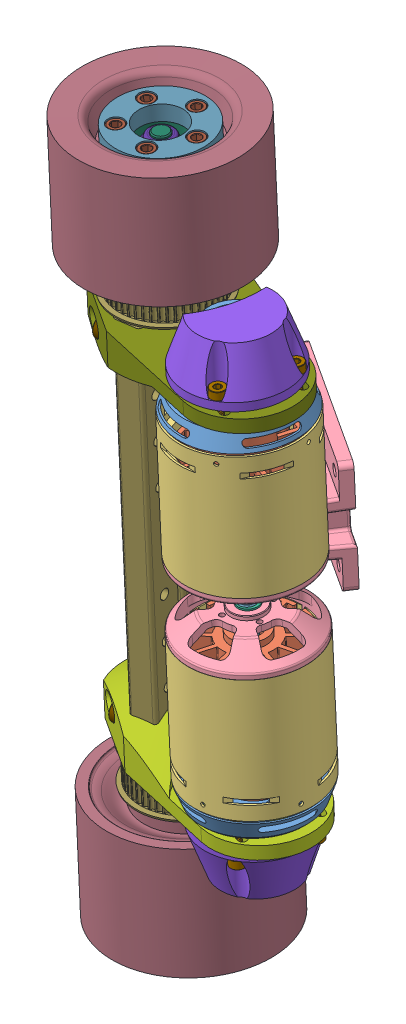
SolidWorks assembly MBS trucks, configuration Default. Lengths in mm.
Overall size (186.8 351.93 169.98).
89 component instances, 34 part files, 94 mates.
Components (placement in the parent):
- GPA26GT3150-A-N8-2: GPA26GT3150-A-N8 [Default] at (26.5522 -42.4742 -58.9865) x (-0.019038 0.999391 0.029249) z (0.77019 0.033313 -0.636944) size (20 28 28)
  - GPA26GT3150-A-N8_b-1: GPA26GT3150-A-N8_b [Default] at origin size (20 28 28)
  - SET-SCREW4-3-1: SET-SCREW4-3 [Default] at (10 5.4 0) x (0 -1 0) z (-1 0 0) size (3 4 4)
  - SET-SCREW4-3-2: SET-SCREW4-3 [Default] at (10 -2.2723 -3.2919) x (0 0.568065 0.822984) z (-1 0 0) size (3 4 4)
- Key20mm-2: Key20mm [Default] at (29.2375 -42.4492 -58.093) x (-0.77019 -0.033313 0.636944) z (-0.63753 0.010401 -0.770355) size (3 20 3)
- MarkIITrucksCustomHanger-1: MarkIITrucksCustomHanger [Default] at (-31.1638 36.2817 -181.4556) x (-0.019038 0.999391 0.029249) z (0.838104 0 0.54551) size (348 118.71 110.67)
  - 50cal_baseplateEDIT-1: 50cal_baseplateEDIT [Default] at (40.8754 28.4427 48.4148) size (55.88 41.6 78.53)
  - BS_bushing-1: BS_bushing [Default] at (40.8754 74.2758 55.8381) x (0.903515 -0.328294 -0.275471) z (-0.428557 -0.692132 -0.580768) size (24.64 14.73 24.64)
  - BS_washer-1: BS_washer [Default] at (40.8754 63.8267 68.2909) x (0.781233 0.478195 0.401253) z (-0.624239 0.59846 0.502167) size (29.08 4.06 29.08)
  - kingpin-1: kingpin [Default] at (40.8754 51.905 82.4986) x (0.057682 0.764769 0.641717) z (0.998335 -0.044187 -0.037077) size (16.06 70.1 13.91)
  - kingpin-nut-1: kingpin-nut [90630A115] at (40.8754 87.1097 40.5433) x (0.976709 0.16437 0.137923) z (-0.214569 0.748202 0.627816) size (12.7 8.97 14.66)
  - Pivot_cup-1: Pivot_cup [Default] at (40.8754 44.9216 26.2393) x (-0.987309 0.102082 -0.121656) z (0.158811 0.63463 -0.756323) size (17.46 19.05 17.46)
  - RS_bushing-1: RS_bushing [Default] at (40.8754 76.7422 52.8988) x (0.999722 0.018072 0.015164) z (-0.023591 0.765831 0.642609) size (24.77 14.61 24.77)
  - washer-1: washer [Default] at (171.3754 88.007 62.3923) x (0 0.98686 -0.161575) z (0 0.161575 0.98686) size (11 1 11)
  - BS_washer-2: BS_washer [Default] at (40.8754 87.1097 40.5433) x (-0.947616 0.244683 0.205314) z (0.319411 0.725916 0.609116) size (29.08 4.06 29.08)
  - washer-2: washer [Default] at (196.6254 88.007 62.3923) x (0 -0.726217 0.687466) z (0 -0.687466 -0.726217) size (11 1 11)
  - CustomHanger-1: CustomHanger [Default] at (40.8754 81.1126 56.6072) x (1 0 0) z (0 -0.642788 0.766044) size (253 93.96 18)
  - KegelWheelAssembly-1: KegelWheelAssembly [Default] at (208.2287 131.5766 17.5506) x (0 0.867364 -0.497674) z (0 0.497674 0.867364) size (80 56 80)
    - Kegel 80mm longboard wheel-1: Kegel 80mm longboard wheel [Default] at (-60.1073 30.6906 17.2106) size (80 56 80)
    - 608-bearing-1: 608-bearing [6661K82] at (-60.1073 32.8534 17.2106) x (1 0 0) z (0 -1 0) size (22 22 7)
    - 608-bearing-2: 608-bearing [6661K82] at (-60.1073 15.6034 17.2106) x (-0.561464 0 0.827501) z (0 -1 0) size (22 22 7)
  - FPSSFJAD-D10-L64-T36-Q8-1: FPSSFJAD-D10-L64-T36-Q8 [Default] at (106.8754 88.007 62.3923) x (1 0 0) z (0 -0.232371 0.972627) size (100 10 10)
  - SetScrew_SAE_10-32x.5in-1: SetScrew_SAE_10-32x.5in [92313A829] at (130.8754 96.8695 69.8289) x (0.758718 0.418725 -0.499016) z (0 0.766044 0.642788) size (4.96 4.83 13.07)
  - SetScrew_SAE_10-32x.5in-3: SetScrew_SAE_10-32x.5in [92313A829] at (130.8736 79.1457 54.9542) x (0.758718 0.418725 -0.499016) z (0 -0.766044 -0.642788) size (4.96 4.83 13.07)
  - NylonLockNut_5.16-24-1: NylonLockNut_5.16-24 [97135A225] at (197.1254 88.007 62.3923) x (0 0.323657 0.946174) z (0 0.946174 -0.323657) size (12.7 8.97 14.66)
  - KegelWheelAssembly-3: KegelWheelAssembly [Default] at (-126.478 148.7071 47.4063) x (0 0.867364 -0.497674) z (0 -0.497674 -0.867364) size (80 56 80)
    - Kegel 80mm longboard wheel-1: Kegel 80mm longboard wheel [Default] at (-60.1073 30.6906 17.2106) size (80 56 80)
    - 608-bearing-1: 608-bearing [6661K82] at (-60.1073 32.8534 17.2106) x (1 0 0) z (0 -1 0) size (22 22 7)
    - 608-bearing-2: 608-bearing [6661K82] at (-60.1073 15.6034 17.2106) x (-0.561464 0 0.827501) z (0 -1 0) size (22 22 7)
  - FPSSFJAD-D10-L64-T36-Q8-3: FPSSFJAD-D10-L64-T36-Q8 [Default] at (-25.1246 88.007 62.3923) x (-1 0 0) z (0 0.232371 -0.972627) size (100 10 10)
  - NylonLockNut_5.16-24-3: NylonLockNut_5.16-24 [97135A225] at (-115.3746 88.007 62.3923) x (0 -0.323657 -0.946174) z (0 0.946174 -0.323657) size (12.7 8.97 14.66)
  - SetScrew_SAE_10-32x.5in-7: SetScrew_SAE_10-32x.5in [92313A829] at (-49.1228 96.8708 69.8273) x (-0.758718 0.418725 -0.499016) z (0 0.766044 0.642788) size (4.96 4.83 13.07)
  - SetScrew_SAE_10-32x.5in-8: SetScrew_SAE_10-32x.5in [92313A829] at (-49.1246 79.1444 54.9557) x (-0.758718 0.418725 -0.499016) z (0 -0.766044 -0.642788) size (4.96 4.83 13.07)
- 91274A172_COATED ALLOY STEEL SOCKET HEAD CAP SCREW-1: 91274A172_COATED ALLOY STEEL SOCKET HEAD CAP SCREW [91274A172] at (-10.1778 -9.516 -60.2635) x (0.117443 0.107613 0.987232) z (0.992459 0.022433 -0.12051) size (9.53 9.53 32.48)
- 91274A172_COATED ALLOY STEEL SOCKET HEAD CAP SCREW-2: 91274A172_COATED ALLOY STEEL SOCKET HEAD CAP SCREW [91274A172] at (-14.1739 -8.6338 -93.0088) x (-0.014856 -0.953854 -0.299902) z (0.992459 0.022433 -0.12051) size (9.53 9.53 32.48)
- 91274A172_COATED ALLOY STEEL SOCKET HEAD CAP SCREW-7: 91274A172_COATED ALLOY STEEL SOCKET HEAD CAP SCREW [91274A172] at (-13.3571 157.3822 -55.3789) x (-0.122553 0.160599 -0.979382) z (0.992459 0.022433 -0.12051) size (9.53 9.53 32.48)
- Turnigy6374-6: Turnigy6374 [Default] at (18.5878 -4.184 -56.238) x (0.309684 0.03371 -0.950242) z (-0.950649 -0.009033 -0.310137) size (83.4 113.65 83.4)
  - Stator-1: Stator [Default] at (3.7873 1.8989 -6.3731) size (58.75 9.22 58.75)
  - StatorPart2-1: StatorPart2 [Default] at (3.7873 -16.3511 -6.3731) size (50 66 50)
  - AxelHoldCover-1: AxelHoldCover [Default] at (3.7873 -60.8511 -6.3731) x (0.982235 0 -0.187653) z (0.187653 0 0.982235) size (59.15 61.5 59.15)
  - AxelHold-1: AxelHold [Default] at (3.7873 -60.8511 -6.3731) x (0.729158 0 0.684345) z (0.684345 0 -0.729158) size (59 18.5 59)
  - AxisCust-1: AxisCust [Default] at (3.7873 -73.3511 -6.3731) x (0.844889 0 -0.534942) z (0.534942 0 0.844889) size (8 113.65 8)
  - 90967A120_STAINLESS STEEL EXTERNAL RETAINING RING-1: 90967A120_STAINLESS STEEL EXTERNAL RETAINING RING [90967A120] at (3.7873 12.2489 -6.3731) x (0 -1 0) z (0 0 1) size (0.8 12.1 9.85)
  - 90967A120_STAINLESS STEEL EXTERNAL RETAINING RING-2: 90967A120_STAINLESS STEEL EXTERNAL RETAINING RING [90967A120] at (3.7873 -73.7511 -6.3731) x (0 -1 0) z (-0.841191 0 -0.540738) size (0.8 12.1 9.85)
- MotorMountLeft-3: MotorMountLeft [Default] at (-25.8025 -21.8807 -75.3183) x (-0.019038 0.999391 0.029249) z (-0.309684 -0.03371 0.950242) size (25.4 116.05 69.01)
- Belt Cap Wheel Side - Motor-2: Belt Cap Wheel Side - Motor [Default] at (26.1505 -21.387 -58.3693) x (-0.309684 -0.03371 0.950242) z (0.950649 0.009033 0.310137) size (50.8 25 40.64)
- M4x16mm_BlackZincSteel-3: M4x16mm_BlackZincSteel [91274A119] at (45.5282 -8.7294 -67.976) x (0.992084 0.022514 -0.123538) z (-0.019038 0.999391 0.029249) size (7 7 20.35)
- M4x16mm_BlackZincSteel-4: M4x16mm_BlackZincSteel [91274A119] at (35.8931 -9.7782 -38.4114) x (0.992084 0.022514 -0.123538) z (-0.019038 0.999391 0.029249) size (7 7 20.35)
- 92125A192_TYPE 18-8 SS FLAT-HEAD SOCKET CAP SCREW-9: 92125A192_TYPE 18-8 SS FLAT-HEAD SOCKET CAP SCREW [92125A192] at (16.1756 -20.8033 -77.9703) x (-0.507945 -0.034866 0.860683) z (0.019038 -0.999391 -0.029249) size (8 8 12.4)
- 92125A192_TYPE 18-8 SS FLAT-HEAD SOCKET CAP SCREW-10: 92125A192_TYPE 18-8 SS FLAT-HEAD SOCKET CAP SCREW [92125A192] at (6.5405 -21.8521 -48.4057) x (0.99191 0.022552 -0.124927) z (0.019038 -0.999391 -0.029249) size (8 8 12.4)
- 91251A355_BLACK-OXIDE ALLOY STEEL SOCKET HEAD CAP SCREW-11: 91251A355_BLACK-OXIDE ALLOY STEEL SOCKET HEAD CAP SCREW [91251A355] at (-23.2576 -26.4129 -91.1172) x (0.999816 0.019099 -0.00181) z (-0.019038 0.999391 0.029249) size (7.92 7.92 68.91)
- GPA50GT3150-A-H26_b-1: GPA50GT3150-A-H26_b [Default] at (-25.7787 -23.1299 -75.3548) x (0.019038 -0.999391 -0.029249) z (0.987808 0.01428 0.155018) size (20 51 51)
- Wheel Spacer 2-3: Wheel Spacer 2 [Default] at (-25.0284 -62.5187 -76.5076) x (-0.158306 0.025873 -0.987051) z (0.987207 0.023422 -0.157717) size (44 14.02 44)
- Wheel Spacer Alum-3: Wheel Spacer Alum [Default] at (-25.0284 -62.5187 -76.5076) x (-0.158306 0.025873 -0.987051) z (0.987207 0.023422 -0.157717) size (44 7.62 44)
- 91251A355_BLACK-OXIDE ALLOY STEEL SOCKET HEAD CAP SCREW-12: 91251A355_BLACK-OXIDE ALLOY STEEL SOCKET HEAD CAP SCREW [91251A355] at (-39.8403 -26.9769 -82.6391) x (0.306709 0.033682 -0.951207) z (-0.019038 0.999391 0.029249) size (7.92 7.92 68.91)
- 91251A355_BLACK-OXIDE ALLOY STEEL SOCKET HEAD CAP SCREW-13: 91251A355_BLACK-OXIDE ALLOY STEEL SOCKET HEAD CAP SCREW [91251A355] at (-36.8906 -27.459 -64.2475) x (-0.81026 0.001717 -0.586069) z (-0.019038 0.999391 0.029249) size (7.92 7.92 68.91)
- 91251A355_BLACK-OXIDE ALLOY STEEL SOCKET HEAD CAP SCREW-14: 91251A355_BLACK-OXIDE ALLOY STEEL SOCKET HEAD CAP SCREW [91251A355] at (-18.485 -27.1929 -61.3591) x (-0.807477 -0.03262 0.588997) z (-0.019038 0.999391 0.029249) size (7.92 7.92 68.91)
- 91251A355_BLACK-OXIDE ALLOY STEEL SOCKET HEAD CAP SCREW-15: 91251A355_BLACK-OXIDE ALLOY STEEL SOCKET HEAD CAP SCREW [91251A355] at (-10.0593 -26.5464 -77.9655) x (0.311212 -0.021878 0.950089) z (-0.019038 0.999391 0.029249) size (7.92 7.92 68.91)
- Wheel Spacer-3: Wheel Spacer [Default] at (-25.0284 -62.5187 -76.5076) x (0.154506 0.031844 -0.987479) z (0.987808 0.01428 0.155018) size (44 7.02 44)
- 91274A172_COATED ALLOY STEEL SOCKET HEAD CAP SCREW-8: 91274A172_COATED ALLOY STEEL SOCKET HEAD CAP SCREW [91274A172] at (-13.3571 157.3822 -55.3789) x (-0.122553 0.160599 -0.979382) z (0.992459 0.022433 -0.12051) size (9.53 9.53 32.48)
- 91274A172_COATED ALLOY STEEL SOCKET HEAD CAP SCREW-9: 91274A172_COATED ALLOY STEEL SOCKET HEAD CAP SCREW [91274A172] at (-17.3532 158.2645 -88.1242) x (0.051476 -0.968499 0.24364) z (0.992459 0.022433 -0.12051) size (9.53 9.53 32.48)
- Turnigy6374-7: Turnigy6374 [Default] at (27.7121 153.0376 -47.6869) x (0.309684 0.03371 -0.950242) z (0.950649 0.009033 0.310137) size (83.4 113.65 83.4)
  - Stator-1: Stator [Default] at (3.7873 1.8989 -6.3731) size (58.75 9.22 58.75)
  - StatorPart2-1: StatorPart2 [Default] at (3.7873 -16.3511 -6.3731) size (50 66 50)
  - AxelHoldCover-1: AxelHoldCover [Default] at (3.7873 -60.8511 -6.3731) x (0.982235 0 -0.187653) z (0.187653 0 0.982235) size (59.15 61.5 59.15)
  - AxelHold-1: AxelHold [Default] at (3.7873 -60.8511 -6.3731) x (0.729158 0 0.684345) z (0.684345 0 -0.729158) size (59 18.5 59)
  - AxisCust-1: AxisCust [Default] at (3.7873 -73.3511 -6.3731) x (0.844889 0 -0.534942) z (0.534942 0 0.844889) size (8 113.65 8)
  - 90967A120_STAINLESS STEEL EXTERNAL RETAINING RING-1: 90967A120_STAINLESS STEEL EXTERNAL RETAINING RING [90967A120] at (3.7873 12.2489 -6.3731) x (0 -1 0) z (0 0 1) size (0.8 12.1 9.85)
  - 90967A120_STAINLESS STEEL EXTERNAL RETAINING RING-2: 90967A120_STAINLESS STEEL EXTERNAL RETAINING RING [90967A120] at (3.7873 -73.7511 -6.3731) x (0 -1 0) z (-0.841191 0 -0.540738) size (0.8 12.1 9.85)
- Belt Cap Wheel Side - Motor-3: Belt Cap Wheel Side - Motor [Default] at (22.4952 170.496 -52.7534) x (0.309684 0.03371 -0.950242) z (0.950649 0.009033 0.310137) size (50.8 25 40.64)
- M4x16mm_BlackZincSteel-5: M4x16mm_BlackZincSteel [91274A119] at (42.3298 159.1682 -63.0621) x (0.992084 0.022514 -0.123538) z (0.019038 -0.999391 -0.029249) size (7 7 20.35)
- M4x16mm_BlackZincSteel-6: M4x16mm_BlackZincSteel [91274A119] at (32.6947 158.1194 -33.4975) x (0.992084 0.022514 -0.123538) z (0.019038 -0.999391 -0.029249) size (7 7 20.35)
- 92125A192_TYPE 18-8 SS FLAT-HEAD SOCKET CAP SCREW-11: 92125A192_TYPE 18-8 SS FLAT-HEAD SOCKET CAP SCREW [92125A192] at (12.5279 170.68 -72.3661) x (0.507945 0.034866 -0.860683) z (-0.019038 0.999391 0.029249) size (8 8 12.4)
- 92125A192_TYPE 18-8 SS FLAT-HEAD SOCKET CAP SCREW-12: 92125A192_TYPE 18-8 SS FLAT-HEAD SOCKET CAP SCREW [92125A192] at (2.8928 169.6312 -42.8016) x (0.99191 0.022552 -0.124927) z (-0.019038 0.999391 0.029249) size (8 8 12.4)
- 91251A355_BLACK-OXIDE ALLOY STEEL SOCKET HEAD CAP SCREW-16: 91251A355_BLACK-OXIDE ALLOY STEEL SOCKET HEAD CAP SCREW [91251A355] at (-27.1048 175.544 -85.2065) x (0.999816 0.019099 -0.00181) z (0.019038 -0.999391 -0.029249) size (7.92 7.92 68.91)
- GPA50GT3150-A-H26_b-2: GPA50GT3150-A-H26_b [Default] at (-29.4816 171.2516 -69.6658) x (-0.019038 0.999391 0.029249) z (-0.987808 -0.01428 -0.155018) size (20 51 51)
- Wheel Spacer 2-4: Wheel Spacer 2 [Default] at (-30.2319 210.6404 -68.513) x (0.158306 -0.025873 0.987051) z (0.987207 0.023422 -0.157717) size (44 14.02 44)
- Wheel Spacer Alum-4: Wheel Spacer Alum [Default] at (-30.2319 210.6404 -68.513) x (0.158306 -0.025873 0.987051) z (0.987207 0.023422 -0.157717) size (44 7.62 44)
- Wheel Spacer-4: Wheel Spacer [Default] at (-30.2319 210.6404 -68.513) x (0.154506 0.031844 -0.987479) z (-0.987808 -0.01428 -0.155018) size (44 7.02 44)
- GPA26GT3150-A-N8-3: GPA26GT3150-A-N8 [Default] at (22.4742 171.5953 -52.7212) x (-0.019038 0.999391 0.029249) z (0.77019 0.033313 -0.636944) size (20 28 28)
  - GPA26GT3150-A-N8_b-1: GPA26GT3150-A-N8_b [Default] at origin size (20 28 28)
  - SET-SCREW4-3-1: SET-SCREW4-3 [Default] at (10 5.4 0) x (0 -1 0) z (-1 0 0) size (3 4 4)
  - SET-SCREW4-3-2: SET-SCREW4-3 [Default] at (10 -2.2723 -3.2919) x (0 0.568065 0.822984) z (-1 0 0) size (3 4 4)
- Key20mm-3: Key20mm [Default] at (26.6914 191.5769 -48.9317) x (-0.77019 -0.033313 0.636944) z (0.63753 -0.010401 0.770355) size (3 20 3)
- MotorMountRight-2: MotorMountRight [Default] at (-29.4578 170.0024 -69.7024) x (-0.019038 0.999391 0.029249) z (-0.309684 -0.03371 0.950242) size (25.4 116.05 69.01)
- 91251A355_BLACK-OXIDE ALLOY STEEL SOCKET HEAD CAP SCREW-17: 91251A355_BLACK-OXIDE ALLOY STEEL SOCKET HEAD CAP SCREW [91251A355] at (-13.9065 175.4105 -72.0548) x (-0.311212 0.021878 -0.950089) z (0.019038 -0.999391 -0.029249) size (7.92 7.92 68.91)
- 91251A355_BLACK-OXIDE ALLOY STEEL SOCKET HEAD CAP SCREW-18: 91251A355_BLACK-OXIDE ALLOY STEEL SOCKET HEAD CAP SCREW [91251A355] at (-22.3322 174.764 -55.4484) x (-0.807477 -0.03262 0.588997) z (0.019038 -0.999391 -0.029249) size (7.92 7.92 68.91)
- 91251A355_BLACK-OXIDE ALLOY STEEL SOCKET HEAD CAP SCREW-19: 91251A355_BLACK-OXIDE ALLOY STEEL SOCKET HEAD CAP SCREW [91251A355] at (-40.7378 174.4979 -58.3368) x (-0.81026 0.001717 -0.586069) z (0.019038 -0.999391 -0.029249) size (7.92 7.92 68.91)
- 91251A355_BLACK-OXIDE ALLOY STEEL SOCKET HEAD CAP SCREW-20: 91251A355_BLACK-OXIDE ALLOY STEEL SOCKET HEAD CAP SCREW [91251A355] at (-43.6875 174.98 -76.7283) x (-0.306709 -0.033682 0.951207) z (0.019038 -0.999391 -0.029249) size (7.92 7.92 68.91)
Mates (geometry in assembly coordinates):
- Concentric1: concentric anti-aligned: cylinder of ? through (0 89.5 0) axis (0 -1 0) radius 6; cylinder of ? through (0 92.55 0) axis (0 1 0) radius 6
- Concentric2: concentric anti-aligned: cylinder of ? through (0 -26.5 0) axis (0 1 0) radius 4; cylinder of GPA26GT3150-A-N8-2/GPA26GT3150-A-N8_b-1 through (0 -6.5 0) axis (0 -1 0) radius 4
- Coincident1: coincident aligned: plane of ? through (0 -26.5 0) normal (0 -1 0); plane of GPA26GT3150-A-N8-2/GPA26GT3150-A-N8_b-1 through (0 -26.5 0) normal (0 -1 0)
- Coincident7: coincident anti-aligned: line of ? through (-1.5 -26.5 -2.5) axis (0 0 -1); line of GPA26GT3150-A-N8-2/GPA26GT3150-A-N8_b-1 through (-1.5 -26.5 -5.4) axis (0 0 1)
- Coincident8: coincident aligned: plane of GPA26GT3150-A-N8-2/GPA26GT3150-A-N8_b-1 through (26.5522 -42.4742 -58.9865) normal (0.019038 -0.999391 -0.029249); plane of Key20mm-2 through (29.2375 -42.4492 -58.093) normal (0.019038 -0.999391 -0.029249)
- Coincident9: coincident anti-aligned: plane of ? through (1.5 -6.5 -2.5) normal (0 0 -1); plane of Key20mm-2 through (-1.5 -6.5 -2.5) normal (0 0 1)
- Coincident10: coincident anti-aligned: plane of GPA26GT3150-A-N8-2/GPA26GT3150-A-N8_b-1 through (30.7694 -22.4926 -55.197) normal (-0.77019 -0.033313 0.636944); plane of Key20mm-2 through (28.8568 -22.4614 -57.508) normal (0.77019 0.033313 -0.636944)
- Concentric5: concentric anti-aligned: cylinder of MarkIITrucksCustomHanger-1/CustomHanger-1 through (-77.4086 -5.45 -20.7444) axis (0 -1 0) radius 9; cylinder of ? through (-77.4086 -27.45 -20.7444) axis (0 1 0) radius 11
- Coincident15: coincident anti-aligned: plane of ? through (-77.2299 -26.5 -21.3999) normal (0 1 0); plane of ? through (-51.5162 -26.5 -25.2476) normal (0 -1 0)
- Coincident28: coincident anti-aligned: plane of MarkIITrucksCustomHanger-1/CustomHanger-1; plane of ? through (-34.0921 -14.7886 -63.0299) normal (-0.017088 0 -0.999854)
- Coincident37: coincident aligned: plane of ? through (-44.2534 59.243 -27.1128) normal (-0.40707 0 0.913397); plane of ? through (38.0802 32.893 9.5804) normal (-0.40707 0 0.913397)
- Coincident38: coincident anti-aligned: plane of ? through (-30.006 52.893 -59.0817) normal (0 -1 0); plane of ? through (52.3276 52.893 -22.3885) normal (0 1 0)
- Coincident40: coincident anti-aligned: plane of ? through (0 0 0) normal (0 -1 0); plane of ? through (-73.3266 0 -32.3363) normal (0 1 0)
- Concentric12: concentric aligned: cylinder of ? through (0 -26.5 0) axis (0 1 0) radius 4; cylinder of ? through (0 -6.35 0) axis (0 1 0) radius 6
- Coincident41: coincident anti-aligned: plane of ?; plane of ? through (-51.7284 -27.45 -24.8099) normal (0 -1 0)
- Concentric17: concentric aligned: cylinder of MarkIITrucksCustomHanger-1/CustomHanger-1 through (-34.2459 -20.2386 -72.0286) axis (0 -1 0) radius 9; cylinder of ? through (-34.2459 -22.2386 -72.0286) axis (0 -1 0) radius 10
- Coincident43: coincident anti-aligned: plane of ?; plane of ? through (-34.2459 -42.2386 -72.0286) normal (0 -1 0)
- Concentric18: concentric anti-aligned: cylinder of ? through (-93.4436 208.55 -19.2392) axis (0 -1 0) radius 2.54; cylinder of ? through (-93.4436 193.63 -19.2392) axis (0 1 0) radius 2.413
- Coincident45: coincident anti-aligned: plane of ? through (-93.4436 193.63 -19.2392) normal (0 -1 0); plane of ? through (-93.4436 193.63 -19.2392) normal (0 1 0)
- Concentric19: concentric: cylinder of ? through (-93.4436 208.55 -19.2392) axis (0 -1 0) radius 2.54; cylinder of ? through (-93.4436 193.63 -19.2392) axis (0 1 0) radius 2.413
- Coincident47: coincident anti-aligned: plane of ? through (-93.4436 193.63 -19.2392) normal (0 -1 0); plane of ? through (-93.4436 193.63 -19.2392) normal (0 1 0)
- Coincident48: coincident anti-aligned: plane of ? through (-29.8766 191.989 -69.0589) normal (0.019038 -0.999391 -0.029249); plane of ? through (-43.0816 192.3928 -91.4524) normal (-0.019038 0.999391 0.029249)
- Concentric28: concentric anti-aligned: cylinder of ? through (-15.3407 192.0809 -62.7407) axis (-0.019038 0.999391 0.029249) radius 2.9; cylinder of ? through (-16.2508 239.8547 -61.3425) axis (0.019038 -0.999391 -0.029249) radius 2.413
- Coincident56: coincident anti-aligned: plane of GPA26GT3150-A-N8-2/GPA26GT3150-A-N8_b-1 through (28.4588 -22.5925 -53.2861) normal (-0.63753 0.010401 -0.770355); plane of Key20mm-2 through (30.7694 -22.4926 -55.197) normal (0.63753 -0.010401 0.770355)
- Coincident58: coincident aligned: plane of GPA26GT3150-A-N8-2/GPA26GT3150-A-N8_b-1; plane of ? through (-22.9313 -22.2386 -48.6196) normal (0 1 0)
- Concentric38: concentric aligned: cylinder of MarkIITrucksCustomHanger-1/CustomHanger-1 through (-41.8828 -7.7386 -55.3957) axis (0.999854 0 -0.017088) radius 2.3813; cylinder of ? through (-80.4696 -7.7386 -54.7362) axis (0.999854 0 -0.017088) radius 5
- Concentric40: concentric aligned: cylinder of ? through (-81.0335 -7.7386 -87.7314) axis (0.999854 0 -0.017088) radius 5; cylinder of 91274A172_COATED ALLOY STEEL SOCKET HEAD CAP SCREW-2 through (-52.2253 -7.7386 -88.2237) axis (0.999854 0 -0.017088) radius 4.7625
- Concentric41: concentric aligned: cylinder of ? through (-80.4696 -7.7386 -54.7362) axis (0.999854 0 -0.017088) radius 5; cylinder of 91274A172_COATED ALLOY STEEL SOCKET HEAD CAP SCREW-1 through (-51.6614 -7.7386 -55.2286) axis (0.999854 0 -0.017088) radius 4.7625
- Coincident61: coincident anti-aligned: plane of ? through (-45.3123 -7.7386 -55.3371) normal (-0.999854 0 0.017088); plane of 91274A172_COATED ALLOY STEEL SOCKET HEAD CAP SCREW-1 through (-45.3123 -7.7386 -55.3371) normal (0.999854 0 -0.017088)
- Coincident62: coincident anti-aligned: plane of ? through (-45.8762 -7.7386 -88.3322) normal (-0.999854 0 0.017088); plane of 91274A172_COATED ALLOY STEEL SOCKET HEAD CAP SCREW-2 through (-45.8762 -7.7386 -88.3322) normal (0.999854 0 -0.017088)
- Coincident65: coincident anti-aligned: plane of MarkIITrucksCustomHanger-1/CustomHanger-1; plane of ? through (-40.595 4.2614 -71.9201) normal (0.999854 0 -0.017088)
- Coincident68: coincident anti-aligned: plane of ? through (-34.2459 -14.7886 -72.0286) normal (0 1 0); plane of Turnigy6374-6/Stator-1 through (52.6547 -14.7886 -33.3) normal (0 -1 0)
- Concentric46: concentric anti-aligned: cylinder of GPA26GT3150-A-N8-2/GPA26GT3150-A-N8_b-1 through (26.1714 -22.4864 -58.4015) axis (0.019038 -0.999391 -0.029249) radius 4; cylinder of Turnigy6374-6/AxisCust-1 through (26.536 -41.6247 -58.9616) axis (-0.019038 0.999391 0.029249) radius 4
- Coincident70: coincident anti-aligned: plane of Key20mm-2 through (28.8568 -22.4614 -57.508) normal (0.77019 0.033313 -0.636944); plane of Turnigy6374-6/AxisCust-1 through (30.8331 -22.4936 -55.1199) normal (-0.77019 -0.033313 0.636944)
- Concentric55: concentric aligned: cylinder of 91274A172_COATED ALLOY STEEL SOCKET HEAD CAP SCREW-1 through (-51.6614 -7.7386 -55.2286) axis (0.999854 0 -0.017088) radius 4.7625; cylinder of ? through (-80.4696 -7.7386 -54.7362) axis (0.999854 0 -0.017088) radius 3.175
- Coincident75: coincident anti-aligned: plane of 91274A172_COATED ALLOY STEEL SOCKET HEAD CAP SCREW-1; plane of ? through (-45.3123 -7.7386 -55.3371) normal (-0.999854 0 0.017088)
- Coincident76: coincident anti-aligned: plane of MarkIITrucksCustomHanger-1/CustomHanger-1; plane of ? through (-40.595 4.2614 -71.9201) normal (0.999854 0 -0.017088)
- Coincident77: coincident anti-aligned: plane of MarkIITrucksCustomHanger-1/CustomHanger-1; plane of ? through (-34.0921 -14.7886 -63.0299) normal (-0.017088 0 -0.999854)
- Concentric56: concentric aligned: cylinder of 91274A172_COATED ALLOY STEEL SOCKET HEAD CAP SCREW-2 through (-54.3819 -7.7386 -88.1869) axis (0.999854 0 -0.017088) radius 4.7625; cylinder of ? through (-81.0335 -7.7386 -87.7314) axis (0.999854 0 -0.017088) radius 5
- Concentric57: concentric aligned: cylinder of MarkIITrucksCustomHanger-1/CustomHanger-1 through (-41.8828 -7.7386 -55.3957) axis (0.999854 0 -0.017088) radius 2.3813; cylinder of ? through (-80.4696 -7.7386 -54.7362) axis (0.999854 0 -0.017088) radius 5
- Concentric58: concentric aligned: cylinder of 91274A172_COATED ALLOY STEEL SOCKET HEAD CAP SCREW-7 through (-51.6614 159.2614 -55.2286) axis (0.999854 0 -0.017088) radius 4.7625; cylinder of ? through (-80.4696 159.2614 -54.7362) axis (0.999854 0 -0.017088) radius 5
- Coincident78: coincident anti-aligned: plane of 91274A172_COATED ALLOY STEEL SOCKET HEAD CAP SCREW-7; plane of ? through (-45.3123 159.2614 -55.3371) normal (-0.999854 0 0.017088)
- Concentric59: concentric aligned: cylinder of 91274A172_COATED ALLOY STEEL SOCKET HEAD CAP SCREW-8 through (-52.2253 159.2614 -88.2237) axis (0.999854 0 -0.017088) radius 4.7625; cylinder of ? through (-81.0335 159.2614 -87.7314) axis (0.999854 0 -0.017088) radius 5
- Coincident79: coincident anti-aligned: plane of MarkIITrucksCustomHanger-1/CustomHanger-1; plane of ? through (-43.2446 -0.6886 -71.8748) normal (0.999854 0 -0.017088)
- Concentric60: concentric anti-aligned: cylinder of 91274A172_COATED ALLOY STEEL SOCKET HEAD CAP SCREW-2 through (-52.2253 -7.7386 -88.2237) axis (0.999854 0 -0.017088) radius 4.7625; circle of ?
- Coincident80: coincident anti-aligned: plane of 91274A172_COATED ALLOY STEEL SOCKET HEAD CAP SCREW-2; plane of ? through (-45.8762 -7.7386 -88.3322) normal (-0.999854 0 0.017088)
- Concentric61: concentric aligned: cylinder of MarkIITrucksCustomHanger-1/CustomHanger-1 through (-35.8988 -9.1248 -90.3708) axis (0.992459 0.022433 -0.12051) radius 2.3813; cylinder of 91274A172_COATED ALLOY STEEL SOCKET HEAD CAP SCREW-2 through (-45.6844 -9.346 -89.1826) axis (0.992459 0.022433 -0.12051) radius 4.7625
- Concentric62: concentric aligned: cylinder of MarkIITrucksCustomHanger-1/CustomHanger-1 through (-41.8828 -7.7386 -55.3957) axis (0.999854 0 -0.017088) radius 2.3813; cylinder of ? through (-80.4696 -7.7386 -54.7362) axis (0.999854 0 -0.017088) radius 3.175
- Concentric63: concentric: cylinder of 91274A172_COATED ALLOY STEEL SOCKET HEAD CAP SCREW-1 through (-51.6614 -7.7386 -55.2286) axis (0.999854 0 -0.017088) radius 4.7625; cylinder of ? through (-80.4696 -7.7386 -54.7362) axis (0.999854 0 -0.017088) radius 5
- Coincident81: coincident anti-aligned: plane of 91274A172_COATED ALLOY STEEL SOCKET HEAD CAP SCREW-1; plane of ? through (-45.3123 -7.7386 -55.3371) normal (-0.999854 0 0.017088)
- Coincident86: coincident aligned: plane of GPA26GT3150-A-N8-2/GPA26GT3150-A-N8_b-1 through (26.5522 -42.4742 -58.9865) normal (0.019038 -0.999391 -0.029249); plane of Turnigy6374-6/AxisCust-1 through (26.5522 -42.4742 -58.9865) normal (0.019038 -0.999391 -0.029249)
- Coincident87: coincident anti-aligned: plane of MarkIITrucksCustomHanger-1/CustomHanger-1; plane of ? through (-33.8358 147.2614 -48.0321) normal (-0.017088 0 -0.999854)
- Concentric72: concentric aligned: cylinder of MarkIITrucksCustomHanger-1/CustomHanger-1 through (-35.0821 156.8912 -52.7409) axis (0.992459 0.022433 -0.12051) radius 2.3813; cylinder of 91274A172_COATED ALLOY STEEL SOCKET HEAD CAP SCREW-7 through (-44.8677 156.67 -51.5527) axis (0.992459 0.022433 -0.12051) radius 4.7625
- Concentric73: concentric aligned: cylinder of 91274A172_COATED ALLOY STEEL SOCKET HEAD CAP SCREW-1 through (-41.6884 -10.2283 -56.4373) axis (0.992459 0.022433 -0.12051) radius 4.7625; cylinder of MotorMountLeft-3 through (-99.4178 -11.5332 -49.4275) axis (0.992459 0.022433 -0.12051) radius 5
- Concentric74: concentric aligned: cylinder of 91274A172_COATED ALLOY STEEL SOCKET HEAD CAP SCREW-2 through (-45.6844 -9.346 -89.1826) axis (0.992459 0.022433 -0.12051) radius 4.7625; cylinder of MotorMountLeft-3 through (-103.4139 -10.6509 -82.1728) axis (0.992459 0.022433 -0.12051) radius 5
- Coincident99: coincident anti-aligned: plane of MarkIITrucksCustomHanger-1/CustomHanger-1 through (-40.1271 204.0204 -76.5538) normal (-0.992459 -0.022433 0.12051); plane of MotorMountLeft-3 through (-34.8555 -15.7364 -74.0479) normal (0.992459 0.022433 -0.12051)
- Coincident100: coincident anti-aligned: plane of 91274A172_COATED ALLOY STEEL SOCKET HEAD CAP SCREW-1 through (-35.3862 -10.0858 -57.2026) normal (0.992459 0.022433 -0.12051); plane of MotorMountLeft-3 through (-35.3862 -10.0858 -57.2026) normal (-0.992459 -0.022433 0.12051)
- Coincident101: coincident anti-aligned: plane of 91274A172_COATED ALLOY STEEL SOCKET HEAD CAP SCREW-2 through (-39.3823 -9.2036 -89.9479) normal (0.992459 0.022433 -0.12051); plane of MotorMountLeft-3 through (-39.3823 -9.2036 -89.9479) normal (-0.992459 -0.022433 0.12051)
- Coincident108: coincident anti-aligned: plane of Turnigy6374-6/Stator-1 through (26.0296 -15.0409 -58.1836) normal (0.019038 -0.999391 -0.029249); plane of MotorMountLeft-3 through (-25.9234 -15.5345 -75.1325) normal (-0.019038 0.999391 0.029249)
- Concentric92: concentric aligned: cylinder of Belt Cap Wheel Side - Motor-2 through (46.2516 -46.7063 -69.0875) axis (-0.019038 0.999391 0.029249) radius 4; cylinder of M4x16mm_BlackZincSteel-3 through (45.9089 -28.7172 -68.561) axis (-0.019038 0.999391 0.029249) radius 3.5
- Concentric93: concentric aligned: cylinder of Belt Cap Wheel Side - Motor-2 through (36.6165 -47.7551 -39.5229) axis (-0.019038 0.999391 0.029249) radius 4; cylinder of M4x16mm_BlackZincSteel-4 through (36.2739 -29.7661 -38.9964) axis (-0.019038 0.999391 0.029249) radius 3.5
- Coincident121: coincident anti-aligned: plane of Belt Cap Wheel Side - Motor-2 through (45.8328 -24.7197 -68.444) normal (0.019038 -0.999391 -0.029249); plane of M4x16mm_BlackZincSteel-3 through (45.8328 -24.7197 -68.444) normal (-0.019038 0.999391 0.029249)
- Coincident122: coincident anti-aligned: plane of Belt Cap Wheel Side - Motor-2 through (36.1977 -25.7685 -38.8794) normal (0.019038 -0.999391 -0.029249); plane of M4x16mm_BlackZincSteel-4 through (36.1977 -25.7685 -38.8794) normal (-0.019038 0.999391 0.029249)
- Coincident123: coincident anti-aligned: plane of MotorMountLeft-3 through (-25.8025 -21.8807 -75.3183) normal (0.019038 -0.999391 -0.029249); plane of Belt Cap Wheel Side - Motor-2 through (26.1505 -21.387 -58.3693) normal (-0.019038 0.999391 0.029249)
- Tangent4: tangent anti-aligned: plane of MotorMountLeft-3 through (-19.5742 -22.104 -94.403) normal (-0.205517 -0.730513 0.65124); cone of ? through (71.8505 -7.1277 -46.5804) axis (-0.019038 0.999391 0.029249)
- Tangent5: tangent anti-aligned: plane of MotorMountLeft-3 through (-29.2093 -23.1528 -64.8384) normal (-0.205517 -0.730513 0.65124); cone of ? through (89.6321 -19.6632 -21.2486) axis (-0.019038 0.999391 0.029249)
- Tangent9: tangent anti-aligned: plane of MotorMountLeft-3 through (-29.2093 -23.1528 -64.8384) normal (-0.205517 -0.730513 0.65124); cone of ? through (89.6321 -19.6632 -21.2486) axis (-0.019038 0.999391 0.029249)
- Tangent10: tangent: plane of MotorMountLeft-3 through (-29.9141 -26.8849 -62.5695) normal (-0.309684 -0.03371 0.950242); curve of ?
- Concentric105: concentric anti-aligned: cylinder of Turnigy6374-6/Stator-1 through (89.3833 -6.6015 -20.8663) axis (0.019038 -0.999391 -0.029249) radius 1.8559; circle of ?
- Concentric106: concentric anti-aligned: cylinder of Turnigy6374-6/Stator-1 through (71.8325 -6.1841 -46.5528) axis (0.019038 -0.999391 -0.029249) radius 1.8559; circle of ?
- Concentric107: concentric anti-aligned: cylinder of Turnigy6374-6/Stator-1 through (45.4602 -5.162 -67.8716) axis (0.019038 -0.999391 -0.029249) radius 1.8559; circle of M4x16mm_BlackZincSteel-3
- Concentric108: concentric anti-aligned: cylinder of Turnigy6374-6/Stator-1 through (35.8251 -6.2108 -38.307) axis (0.019038 -0.999391 -0.029249) radius 1.8559; cylinder of M4x16mm_BlackZincSteel-4 through (36.2739 -29.7661 -38.9964) axis (-0.019038 0.999391 0.029249) radius 3.5
- Tangent18: tangent anti-aligned: plane of MotorMountLeft-3 through (-19.5914 -21.2046 -94.3766) normal (-0.205517 -0.730513 0.65124); cone of 92125A192_TYPE 18-8 SS FLAT-HEAD SOCKET CAP SCREW-9 through (16.1318 -18.5047 -77.9031) axis (-0.019038 0.999391 0.029249)
- Tangent19: tangent anti-aligned: plane of MotorMountLeft-3 through (-31.287 -19.974 -58.5624) normal (0.232441 -0.682839 -0.692605); cone of 92125A192_TYPE 18-8 SS FLAT-HEAD SOCKET CAP SCREW-10 through (6.4967 -19.5535 -48.3385) axis (-0.019038 0.999391 0.029249)
- Concentric109: concentric anti-aligned: cylinder of Turnigy6374-6/Stator-1 through (6.2479 -6.4918 -47.9562) axis (0.019038 -0.999391 -0.029249) radius 1.8559; circle of 92125A192_TYPE 18-8 SS FLAT-HEAD SOCKET CAP SCREW-10
- Concentric110: concentric anti-aligned: cylinder of Turnigy6374-6/Stator-1 through (15.883 -5.443 -77.5208) axis (0.019038 -0.999391 -0.029249) radius 1.8559; circle of 92125A192_TYPE 18-8 SS FLAT-HEAD SOCKET CAP SCREW-9
- Coincident124: coincident aligned: cone of MotorMountLeft-3 through (6.4967 -19.5535 -48.3385) axis (-0.019038 0.999391 0.029249); cone of 92125A192_TYPE 18-8 SS FLAT-HEAD SOCKET CAP SCREW-10 through (6.4967 -19.5535 -48.3385) axis (-0.019038 0.999391 0.029249)
- Coincident140: coincident anti-aligned: plane of ? through (-15.0116 238.8514 -69.4308) normal (0.019038 -0.999391 -0.029249); plane of ? through (-15.0116 238.8514 -69.4308) normal (-0.019038 0.999391 0.029249)
- Concentric122: concentric aligned: cylinder of MotorMountLeft-3 through (45.8261 -24.3699 -68.4338) axis (-0.019038 0.999391 0.029249) radius 2; cylinder of M4x16mm_BlackZincSteel-3 through (45.9089 -28.7172 -68.561) axis (-0.019038 0.999391 0.029249) radius 3.5
- Concentric128: concentric anti-aligned: cylinder of 91251A355_BLACK-OXIDE ALLOY STEEL SOCKET HEAD CAP SCREW-11 through (-21.9568 -94.6973 -93.1157) axis (-0.019038 0.999391 0.029249) radius 3.9624; cylinder of Wheel Spacer Alum-3 through (-22.0487 -89.8742 -92.9746) axis (0.019038 -0.999391 -0.029249) radius 3.9688
- Coincident145: coincident anti-aligned: plane of 91251A355_BLACK-OXIDE ALLOY STEEL SOCKET HEAD CAP SCREW-11 through (-22.0487 -89.8742 -92.9746) normal (-0.019038 0.999391 0.029249); plane of Wheel Spacer Alum-3 through (-22.0487 -89.8742 -92.9746) normal (0.019038 -0.999391 -0.029249)
- Coincident146: coincident aligned: circle of MarkIITrucksCustomHanger-1/KegelWheelAssembly-3/Kegel 80mm longboard wheel-1; circle of Wheel Spacer-3
- Concentric129: concentric aligned: cylinder of MarkIITrucksCustomHanger-1/KegelWheelAssembly-3/Kegel 80mm longboard wheel-1 through (-36.5677 -44.4087 -64.7436) axis (0.019038 -0.999391 -0.029249) radius 2.9; cylinder of Wheel Spacer-3 through (-35.8633 -81.3861 -65.8258) axis (0.019038 -0.999391 -0.029249) radius 2.54
- Coincident147: coincident anti-aligned: plane of Wheel Spacer Alum-3 through (-24.546 -87.8405 -77.2487) normal (-0.019038 0.999391 0.029249); plane of Wheel Spacer-3 through (-24.546 -87.8405 -77.2487) normal (0.019038 -0.999391 -0.029249)
- Concentric130: concentric aligned: circle of Wheel Spacer Alum-3; circle of Wheel Spacer-3
- Concentric131: concentric aligned: circle of Wheel Spacer Alum-3; circle of Wheel Spacer-3
- Concentric132: concentric aligned: cylinder of MarkIITrucksCustomHanger-1/KegelWheelAssembly-3/Kegel 80mm longboard wheel-1 through (-25.3837 -43.8673 -75.9618) axis (-0.019038 0.999391 0.029249) radius 40; cylinder of GPA50GT3150-A-H26_b-1 through (-25.3979 -43.1177 -75.9398) axis (-0.019038 0.999391 0.029249) radius 13
- Coincident148: coincident aligned: circle of MarkIITrucksCustomHanger-1/KegelWheelAssembly-3/Kegel 80mm longboard wheel-1; circle of Wheel Spacer 2-3
- Coincident149: coincident anti-aligned: plane of GPA50GT3150-A-H26_b-1 through (-22.1533 -42.449 -96.6769) normal (0.019038 -0.999391 -0.029249); plane of Wheel Spacer 2-3 through (-25.3979 -43.1177 -75.9398) normal (-0.019038 0.999391 0.029249)
- Concentric133: concentric aligned: cylinder of Wheel Spacer 2-3 through (-39.2651 -57.1685 -83.5227) axis (-0.019038 0.999391 0.029249) radius 2.54; cylinder of 91251A355_BLACK-OXIDE ALLOY STEEL SOCKET HEAD CAP SCREW-12 through (-38.6313 -90.4382 -84.4964) axis (-0.019038 0.999391 0.029249) radius 2.413
- Concentric134: concentric aligned: cylinder of GPA50GT3150-A-H26_b-1 through (-39.5317 -43.177 -83.1132) axis (-0.019038 0.999391 0.029249) radius 2; cylinder of 91251A355_BLACK-OXIDE ALLOY STEEL SOCKET HEAD CAP SCREW-12 through (-38.6313 -90.4382 -84.4964) axis (-0.019038 0.999391 0.029249) radius 2.413
- Coincident154: coincident aligned: plane of MarkIITrucksCustomHanger-1/CustomHanger-1 through (-36.8498 170.1005 -77.8677) normal (-0.019038 0.999391 0.029249); plane of MotorMountRight-2 through (-29.4578 170.0024 -69.7024) normal (-0.019038 0.999391 0.029249)
- Coincident155: coincident anti-aligned: plane of MarkIITrucksCustomHanger-1/CustomHanger-1 through (-22.2628 204.4242 -78.723) normal (0.992459 0.022433 -0.12051); plane of MotorMountRight-2 through (-20.4048 163.8581 -70.9727) normal (-0.992459 -0.022433 0.12051)
- Coincident156: coincident anti-aligned: plane of MarkIITrucksCustomHanger-1/CustomHanger-1 through (-31.026 73.2768 -47.9303) normal (0.121093 -0.026735 0.992281); plane of MotorMountRight-2 through (-26.068 143.9762 -46.6306) normal (-0.121093 0.026735 -0.992281)
